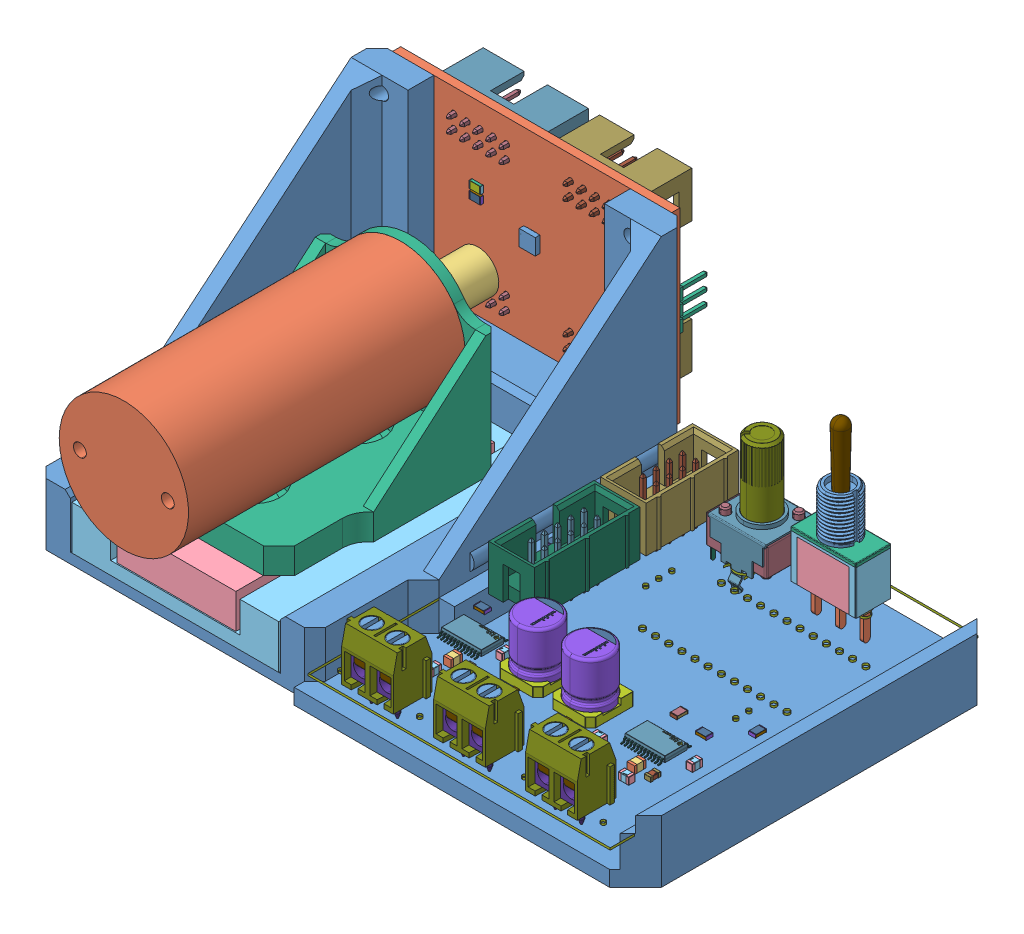
SolidWorks assembly 07_01_00-pidgeon_drive_testing_rig, configuration Default. Lengths in mm.
Overall size (121 48 89.69).
399 component instances, 88 part files, 20 mates.
Components (placement in the parent):
- 07_01_01-encoder_PCB_bracket-1: 07_01_01-encoder_PCB_bracket [Default] at (-11.5568 16.63 42.3747) size (121 48 71)
- 07_01_02-encoder_PCB.step-1: 07_01_02-encoder_PCB.step [Default] at (-14.5568 13.63 42.3747) size (54 36 12.1)
  - Board.step-1: Board.step [Default] at origin size (54 36 1.59)
    - Open CASCADE STEP translator 7.5 1.1.1.step-1: Open CASCADE STEP translator 7.5 1.1.1.step [Default] at (0 0 -1.59) size (54 36 1.59)
  - U2.step-1: U2.step [Default] at origin size (4 3.5 1)
    - 6290729904.step-1: 6290729904.step [Default] at (17.25 17.25 -2.59) size (4 3.5 1)
      - Extruded.step-1: Extruded.step [Default] at origin size (4 3.5 1)
  - R8.step-1: R8.step [Default] at origin size (2.2 1.45 0.7)
    - 6290729184.step-1: 6290729184.step [Default] at (47 19.5 -2.29) size (1.4 1.45 0.7)
      - Extruded-0.step-1: Extruded-0.step [Default] at origin size (1.4 1.45 0.7)
    - 6290729024.step-1: 6290729024.step [Default] at (46.1 19.5 -2.29) size (0.4 1.45 0.7)
      - Extruded-1.step-1: Extruded-1.step [Default] at origin size (0.4 1.45 0.7)
    - 6290729024.step-2: 6290729024.step [Default] at (47.9 19.5 -2.29) size (0.4 1.45 0.7)
      - Extruded-1.step-1: Extruded-1.step [Default] at origin size (0.4 1.45 0.7)
  - R7.step-1: R7.step [Default] at origin size (2.2 1.45 0.7)
    - 6290729184.step-1: 6290729184.step [Default] at (47 17.25 -2.29) size (1.4 1.45 0.7)
      - Extruded-0.step-1: Extruded-0.step [Default] at origin size (1.4 1.45 0.7)
    - 6290729024.step-1: 6290729024.step [Default] at (46.1 17.25 -2.29) size (0.4 1.45 0.7)
      - Extruded-1.step-1: Extruded-1.step [Default] at origin size (0.4 1.45 0.7)
    - 6290729024.step-2: 6290729024.step [Default] at (47.9 17.25 -2.29) size (0.4 1.45 0.7)
      - Extruded-1.step-1: Extruded-1.step [Default] at origin size (0.4 1.45 0.7)
  - R6.step-1: R6.step [Default] at origin size (2.2 1.45 0.7)
    - 6290729184.step-1: 6290729184.step [Default] at (47 15 -2.29) size (1.4 1.45 0.7)
      - Extruded-0.step-1: Extruded-0.step [Default] at origin size (1.4 1.45 0.7)
    - 6290729024.step-1: 6290729024.step [Default] at (46.1 15 -2.29) size (0.4 1.45 0.7)
      - Extruded-1.step-1: Extruded-1.step [Default] at origin size (0.4 1.45 0.7)
    - 6290729024.step-2: 6290729024.step [Default] at (47.9 15 -2.29) size (0.4 1.45 0.7)
      - Extruded-1.step-1: Extruded-1.step [Default] at origin size (0.4 1.45 0.7)
  - P5.step-1: P5.step [Default] at origin size (2.54 7.62 10.92)
    - TSW-103-07-X-S.step-1: TSW-103-07-X-S.step [Default] at (50.7499 18.0199 -1.59) x (0 1 0) z (-1 0 0) size (7.62 10.92 2.54)
  - D3.step-1: D3.step [Default] at origin size (2 1.25 0.8)
    - Diode_Wurth_Electronics_150080SS75000_eec.step-1: Diode_Wurth_Electronics_150080SS75000_eec.step [Default] at (42.5 19.5 -1.59) x (-1 0 0) z (0 0 -1) size (2 1.25 0.8)
      - base.step-1: base.step [Default] at (0.8 0 0) x (-1 0 0) z (0 0 1) size (0.4 1 0.3)
      - cover.step-1: cover.step [Default] at (0 0 0.3) size (1.4 1.25 0.5)
      - housing.step-1: housing.step [Default] at origin size (2 1.25 0.3)
      - marking.step-1: marking.step [Default] at (-0.8 0.525 0.26) size (0.4 0.48 0.04)
      - marking.step-2: marking.step [Default] at (-0.8 -0.525 0.3) x (1 0 0) z (0 0 -1) size (0.4 0.48 0.04)
      - base_2.step-1: base_2.step [Default] at (-0.8 0 0) size (0.4 1 0.3)
      - Mark2.step-1: Mark2.step [Default] at (-0.2 0 0.04) x (-1 0 0) z (0 0 -1) size (0.4 0.46 0)
  - D2.step-1: D2.step [Default] at origin size (2 1.25 0.8)
    - Diode_Wurth_Electronics_150080SS75000_eec.step-1: Diode_Wurth_Electronics_150080SS75000_eec.step [Default] at (42.5 17.25 -1.59) x (-1 0 0) z (0 0 -1) size (2 1.25 0.8)
      - base.step-1: base.step [Default] at (0.8 0 0) x (-1 0 0) z (0 0 1) size (0.4 1 0.3)
      - cover.step-1: cover.step [Default] at (0 0 0.3) size (1.4 1.25 0.5)
      - housing.step-1: housing.step [Default] at origin size (2 1.25 0.3)
      - marking.step-1: marking.step [Default] at (-0.8 0.525 0.26) size (0.4 0.48 0.04)
      - marking.step-2: marking.step [Default] at (-0.8 -0.525 0.3) x (1 0 0) z (0 0 -1) size (0.4 0.48 0.04)
      - base_2.step-1: base_2.step [Default] at (-0.8 0 0) size (0.4 1 0.3)
      - Mark2.step-1: Mark2.step [Default] at (-0.2 0 0.04) x (-1 0 0) z (0 0 -1) size (0.4 0.46 0)
  - D1.step-1: D1.step [Default] at origin size (2 1.25 0.8)
    - Diode_Wurth_Electronics_150080SS75000_eec.step-1: Diode_Wurth_Electronics_150080SS75000_eec.step [Default] at (42.5 15 -1.59) x (-1 0 0) z (0 0 -1) size (2 1.25 0.8)
      - base.step-1: base.step [Default] at (0.8 0 0) x (-1 0 0) z (0 0 1) size (0.4 1 0.3)
      - cover.step-1: cover.step [Default] at (0 0 0.3) size (1.4 1.25 0.5)
      - housing.step-1: housing.step [Default] at origin size (2 1.25 0.3)
      - marking.step-1: marking.step [Default] at (-0.8 0.525 0.26) size (0.4 0.48 0.04)
      - marking.step-2: marking.step [Default] at (-0.8 -0.525 0.3) x (1 0 0) z (0 0 -1) size (0.4 0.48 0.04)
      - base_2.step-1: base_2.step [Default] at (-0.8 0 0) size (0.4 1 0.3)
      - Mark2.step-1: Mark2.step [Default] at (-0.2 0 0.04) x (-1 0 0) z (0 0 -1) size (0.4 0.46 0)
  - C4.step-1: C4.step [Default] at origin size (1.25 2 0.88)
    - Cap_KEMET_C0805C472J3HAC_eec.step-1: Cap_KEMET_C0805C472J3HAC_eec.step [Default] at (25.6247 12.75 -1.59) x (0 -1 0) z (0 0 -1) size (1 1.15 0.78)
    - Cap_KEMET_C0805C472J3HAC_eec-2.step-1: Cap_KEMET_C0805C472J3HAC_eec-2.step [Default] at (25.6247 12.75 -1.59) x (0 -1 0) z (0 0 -1) size (2 1.25 0.88)
    - Cap_KEMET_C0805C472J3HAC_eec-3.step-1: Cap_KEMET_C0805C472J3HAC_eec-3.step [Default] at (25.6247 12.75 -1.59) x (0 -1 0) z (0 0 -1) size (0.59 0.12 0)
  - U4.step-1: U4.step [Default] at origin size (2.8 2.9 1.45)
    - IC_Microchip_MIC7300YM5-TR_eec.step-1: IC_Microchip_MIC7300YM5-TR_eec.step [Default] at (29.5 12.5 -1.59) x (0 -1 0) z (0 0 -1) size (2.9 2.8 1.45)
      - IC_BODY.step-1: IC_BODY.step [Default] at (0 0 0.15) x (0 -1 0) z (0 0 1) size (1.6 2.9 1.3)
      - IC_LEG.step-1: IC_LEG.step [Default] at (1.15 1.4 0) x (0 -1 0) z (-1 0 0) size (0.6 0.86 0.4)
      - IC_LEG.step-2: IC_LEG.step [Default] at (0.2 1.4 0) x (0 -1 0) z (-1 0 0) size (0.6 0.86 0.4)
      - IC_LEG.step-3: IC_LEG.step [Default] at (-0.75 1.4 0) x (0 -1 0) z (-1 0 0) size (0.6 0.86 0.4)
      - circle.step-1: circle.step [Default] at (0.9954 0.3904 1.451) x (1 0 0) z (0 0 -1) size (0.4 0.4 0)
      - IC_LEG_MIR1.step-1: IC_LEG_MIR1.step [Default] at (1.15 -1.4 0) x (0 1 0) z (1 0 0) size (0.6 0.86 0.4)
      - IC_LEG_MIR1.step-2: IC_LEG_MIR1.step [Default] at (-0.75 -1.4 0) x (0 1 0) z (1 0 0) size (0.6 0.86 0.4)
      - Microchip logo.step-1: Microchip logo.step [Default] at (-1.0431 -0.33 1.4496) x (0 -1 0) z (0 0 1) size (0.4 0.39 0)
  - R5.step-1: R5.step [Default] at origin size (2.2 1.45 0.6)
    - 6290728304.step-1: 6290728304.step [Default] at (4.75 23.25 -2.19) size (1.4 1.45 0.6)
      - Extruded-4.step-1: Extruded-4.step [Default] at origin size (1.4 1.45 0.6)
    - 6290728144.step-1: 6290728144.step [Default] at (3.85 23.25 -2.19) size (0.4 1.45 0.6)
      - Extruded-5.step-1: Extruded-5.step [Default] at origin size (0.4 1.45 0.6)
    - 6290728144.step-2: 6290728144.step [Default] at (5.65 23.25 -2.19) size (0.4 1.45 0.6)
      - Extruded-5.step-1: Extruded-5.step [Default] at origin size (0.4 1.45 0.6)
  - R4.step-1: R4.step [Default] at origin size (2.2 1.45 0.6)
    - 6290728304.step-1: 6290728304.step [Default] at (15 23.25 -2.19) size (1.4 1.45 0.6)
      - Extruded-4.step-1: Extruded-4.step [Default] at origin size (1.4 1.45 0.6)
    - 6290728144.step-1: 6290728144.step [Default] at (14.1 23.25 -2.19) size (0.4 1.45 0.6)
      - Extruded-5.step-1: Extruded-5.step [Default] at origin size (0.4 1.45 0.6)
    - 6290728144.step-2: 6290728144.step [Default] at (15.9 23.25 -2.19) size (0.4 1.45 0.6)
      - Extruded-5.step-1: Extruded-5.step [Default] at origin size (0.4 1.45 0.6)
  - R3.step-1: R3.step [Default] at origin size (2.2 1.45 0.6)
    - 6290728304.step-1: 6290728304.step [Default] at (9.25 23.25 -2.19) size (1.4 1.45 0.6)
      - Extruded-4.step-1: Extruded-4.step [Default] at origin size (1.4 1.45 0.6)
    - 6290728144.step-1: 6290728144.step [Default] at (10.15 23.25 -2.19) size (0.4 1.45 0.6)
      - Extruded-5.step-1: Extruded-5.step [Default] at origin size (0.4 1.45 0.6)
    - 6290728144.step-2: 6290728144.step [Default] at (8.35 23.25 -2.19) size (0.4 1.45 0.6)
      - Extruded-5.step-1: Extruded-5.step [Default] at origin size (0.4 1.45 0.6)
  - R2.step-1: R2.step [Default] at origin size (2.2 1.35 0.6)
    - 6361395456.step-1: 6361395456.step [Default] at (16.5 21.75 0) size (2.2 1.35 0.6)
      - Terminal.step-1: Terminal.step [Default] at (-1.1 -0.675 0) size (0.15 1.35 0.6)
        - Open CASCADE STEP translator 6.8 7.2.1.step-1: Open CASCADE STEP translator 6.8 7.2.1.step [Default] at origin size (0.15 1.35 0.6)
      - Terminal.step-2: Terminal.step [Default] at (1.1 0.675 0) x (-1 0 0) z (0 0 1) size (0.15 1.35 0.6)
        - Open CASCADE STEP translator 6.8 7.2.1.step-1: Open CASCADE STEP translator 6.8 7.2.1.step [Default] at origin size (0.15 1.35 0.6)
      - Mid_Body.step-1: Mid_Body.step [Default] at (-1.1 -0.675 0) size (2.08 1.35 0.48)
      - Mark.step-1: Mark.step [Default] at (-0.95 -0.675 0.54) size (1.9 1.35 0.06)
  - R1.step-1: R1.step [Default] at origin size (2.2 1.35 0.6)
    - 6361394336.step-1: 6361394336.step [Default] at (16.5 20 0) x (-1 0 0) z (0 0 1) size (2.2 1.35 0.6)
      - Terminal-1.step-1: Terminal-1.step [Default] at (-1.1 -0.675 0) size (0.15 1.35 0.6)
        - Open CASCADE STEP translator 6.8 7.2.1-6.step-1: Open CASCADE STEP translator 6.8 7.2.1-6.step [Default] at origin size (0.15 1.35 0.6)
      - Terminal-1.step-2: Terminal-1.step [Default] at (1.1 0.675 0) x (-1 0 0) z (0 0 1) size (0.15 1.35 0.6)
        - Open CASCADE STEP translator 6.8 7.2.1-6.step-1: Open CASCADE STEP translator 6.8 7.2.1-6.step [Default] at origin size (0.15 1.35 0.6)
      - Mid_Body-7.step-1: Mid_Body-7.step [Default] at (-1.1 -0.675 0) size (2.08 1.35 0.48)
      - Mark-8.step-1: Mark-8.step [Default] at (-0.95 -0.675 0.54) size (1.9 1.35 0.06)
  - P4.step-1: P4.step [Default] at origin size (17.82 9.18 12.1)
    - 61200821621.step-1: 61200821621.step [Default] at (38.2501 30.2499 -6.29) x (1 0 0) z (0 0 -1) size (17.82 9.17 12.1)
      - 6120xx21621_PIN.step-1: 6120xx21621_PIN.step [Default] at (-0.405 1.27 -1.875) size (0.64 0.64 11.6)
      - 6120xx21621_PIN.step-2: 6120xx21621_PIN.step [Default] at (-0.405 -1.27 -1.875) size (0.64 0.64 11.6)
      - 6120xx21621_PIN.step-3: 6120xx21621_PIN.step [Default] at (2.135 -1.27 -1.875) size (0.64 0.64 11.6)
      - 6120xx21621_PIN.step-4: 6120xx21621_PIN.step [Default] at (4.675 -1.27 -1.875) size (0.64 0.64 11.6)
      - 6120xx21621_PIN.step-5: 6120xx21621_PIN.step [Default] at (2.135 1.27 -1.875) size (0.64 0.64 11.6)
      - 6120xx21621_PIN.step-6: 6120xx21621_PIN.step [Default] at (4.675 1.27 -1.875) size (0.64 0.64 11.6)
      - 6120xx21621_PIN.step-7: 6120xx21621_PIN.step [Default] at (7.215 -1.27 -1.875) size (0.64 0.64 11.6)
      - 6120xx21621_PIN.step-8: 6120xx21621_PIN.step [Default] at (7.215 1.27 -1.875) size (0.64 0.64 11.6)
      - 61200821621-9.step-1: 61200821621-9.step [Default] at origin size (17.82 9.17 9.1)
  - P3.step-1: P3.step [Default] at origin size (20.36 9.18 12.1)
    - 61201021621.step-1: 61201021621.step [Default] at (17.0001 30.2499 -6.29) x (1 0 0) z (0 0 -1) size (20.36 9.17 12.1)
      - 6120xx21621_PIN-10.step-1: 6120xx21621_PIN-10.step [Default] at (-1.675 1.27 -1.875) size (0.64 0.64 11.6)
      - 6120xx21621_PIN-10.step-2: 6120xx21621_PIN-10.step [Default] at (-1.675 -1.27 -1.875) size (0.64 0.64 11.6)
      - 6120xx21621_PIN-10.step-3: 6120xx21621_PIN-10.step [Default] at (0.865 -1.27 -1.875) size (0.64 0.64 11.6)
      - 6120xx21621_PIN-10.step-4: 6120xx21621_PIN-10.step [Default] at (3.405 -1.27 -1.875) size (0.64 0.64 11.6)
      - 6120xx21621_PIN-10.step-5: 6120xx21621_PIN-10.step [Default] at (0.865 1.27 -1.875) size (0.64 0.64 11.6)
      - 6120xx21621_PIN-10.step-6: 6120xx21621_PIN-10.step [Default] at (3.405 1.27 -1.875) size (0.64 0.64 11.6)
      - 6120xx21621_PIN-10.step-7: 6120xx21621_PIN-10.step [Default] at (5.945 -1.27 -1.875) size (0.64 0.64 11.6)
      - 6120xx21621_PIN-10.step-8: 6120xx21621_PIN-10.step [Default] at (5.945 1.27 -1.875) size (0.64 0.64 11.6)
      - 6120xx21621_PIN-10.step-9: 6120xx21621_PIN-10.step [Default] at (8.485 -1.27 -1.875) size (0.64 0.64 11.6)
      - 6120xx21621_PIN-10.step-10: 6120xx21621_PIN-10.step [Default] at (8.485 1.27 -1.875) size (0.64 0.64 11.6)
      - 61201021621-11.step-1: 61201021621-11.step [Default] at origin size (20.36 9.17 9.1)
  - P2.step-1: P2.step [Default] at origin size (17.82 9.18 12.1)
    - 61200821621.step-1: 61200821621.step [Default] at (38.2501 4.9999 -6.29) x (1 0 0) z (0 0 -1) size (17.82 9.17 12.1)
      - 6120xx21621_PIN.step-1: 6120xx21621_PIN.step [Default] at (-0.405 1.27 -1.875) size (0.64 0.64 11.6)
      - 6120xx21621_PIN.step-2: 6120xx21621_PIN.step [Default] at (-0.405 -1.27 -1.875) size (0.64 0.64 11.6)
      - 6120xx21621_PIN.step-3: 6120xx21621_PIN.step [Default] at (2.135 -1.27 -1.875) size (0.64 0.64 11.6)
      - 6120xx21621_PIN.step-4: 6120xx21621_PIN.step [Default] at (4.675 -1.27 -1.875) size (0.64 0.64 11.6)
      - 6120xx21621_PIN.step-5: 6120xx21621_PIN.step [Default] at (2.135 1.27 -1.875) size (0.64 0.64 11.6)
      - 6120xx21621_PIN.step-6: 6120xx21621_PIN.step [Default] at (4.675 1.27 -1.875) size (0.64 0.64 11.6)
      - 6120xx21621_PIN.step-7: 6120xx21621_PIN.step [Default] at (7.215 -1.27 -1.875) size (0.64 0.64 11.6)
      - 6120xx21621_PIN.step-8: 6120xx21621_PIN.step [Default] at (7.215 1.27 -1.875) size (0.64 0.64 11.6)
      - 61200821621-9.step-1: 61200821621-9.step [Default] at origin size (17.82 9.17 9.1)
  - P1.step-1: P1.step [Default] at origin size (20.36 9.18 12.1)
    - 61201021621.step-1: 61201021621.step [Default] at (17.0001 4.9999 -6.29) x (1 0 0) z (0 0 -1) size (20.36 9.17 12.1)
      - 6120xx21621_PIN-10.step-1: 6120xx21621_PIN-10.step [Default] at (-1.675 1.27 -1.875) size (0.64 0.64 11.6)
      - 6120xx21621_PIN-10.step-2: 6120xx21621_PIN-10.step [Default] at (-1.675 -1.27 -1.875) size (0.64 0.64 11.6)
      - 6120xx21621_PIN-10.step-3: 6120xx21621_PIN-10.step [Default] at (0.865 -1.27 -1.875) size (0.64 0.64 11.6)
      - 6120xx21621_PIN-10.step-4: 6120xx21621_PIN-10.step [Default] at (3.405 -1.27 -1.875) size (0.64 0.64 11.6)
      - 6120xx21621_PIN-10.step-5: 6120xx21621_PIN-10.step [Default] at (0.865 1.27 -1.875) size (0.64 0.64 11.6)
      - 6120xx21621_PIN-10.step-6: 6120xx21621_PIN-10.step [Default] at (3.405 1.27 -1.875) size (0.64 0.64 11.6)
      - 6120xx21621_PIN-10.step-7: 6120xx21621_PIN-10.step [Default] at (5.945 -1.27 -1.875) size (0.64 0.64 11.6)
      - 6120xx21621_PIN-10.step-8: 6120xx21621_PIN-10.step [Default] at (5.945 1.27 -1.875) size (0.64 0.64 11.6)
      - 6120xx21621_PIN-10.step-9: 6120xx21621_PIN-10.step [Default] at (8.485 -1.27 -1.875) size (0.64 0.64 11.6)
      - 6120xx21621_PIN-10.step-10: 6120xx21621_PIN-10.step [Default] at (8.485 1.27 -1.875) size (0.64 0.64 11.6)
      - 61201021621-11.step-1: 61201021621-11.step [Default] at origin size (20.36 9.17 9.1)
  - C3.step-1: C3.step [Default] at origin size (1.35 2.1 0.7)
    - 6290729744.step-1: 6290729744.step [Default] at (30 17.75 -2.29) size (1.35 1.2 0.7)
      - Extruded-12.step-1: Extruded-12.step [Default] at origin size (1.35 1.2 0.7)
    - 6290729584.step-1: 6290729584.step [Default] at (30 16.925 -2.29) size (1.35 0.45 0.7)
      - Extruded-13.step-1: Extruded-13.step [Default] at origin size (1.35 0.45 0.7)
    - 6290729584.step-2: 6290729584.step [Default] at (30 18.575 -2.29) size (1.35 0.45 0.7)
      - Extruded-13.step-1: Extruded-13.step [Default] at origin size (1.35 0.45 0.7)
  - C2.step-1: C2.step [Default] at origin size (1.25 2 0.88)
    - Cap_KEMET_C0805C472J3HAC_eec.step-1: Cap_KEMET_C0805C472J3HAC_eec.step [Default] at (2.5 16.25 -1.59) x (0 1 0) z (0 0 -1) size (1 1.15 0.78)
    - Cap_KEMET_C0805C472J3HAC_eec-2.step-1: Cap_KEMET_C0805C472J3HAC_eec-2.step [Default] at (2.5 16.25 -1.59) x (0 1 0) z (0 0 -1) size (2 1.25 0.88)
    - Cap_KEMET_C0805C472J3HAC_eec-3.step-1: Cap_KEMET_C0805C472J3HAC_eec-3.step [Default] at (2.5 16.25 -1.59) x (0 1 0) z (0 0 -1) size (0.59 0.12 0)
  - C1.step-1: C1.step [Default] at origin size (1.25 2 0.88)
    - Cap_KEMET_C0805C472J3HAC_eec.step-1: Cap_KEMET_C0805C472J3HAC_eec.step [Default] at (12.75 16.25 -1.59) x (0 1 0) z (0 0 -1) size (1 1.15 0.78)
    - Cap_KEMET_C0805C472J3HAC_eec-2.step-1: Cap_KEMET_C0805C472J3HAC_eec-2.step [Default] at (12.75 16.25 -1.59) x (0 1 0) z (0 0 -1) size (2 1.25 0.88)
    - Cap_KEMET_C0805C472J3HAC_eec-3.step-1: Cap_KEMET_C0805C472J3HAC_eec-3.step [Default] at (12.75 16.25 -1.59) x (0 1 0) z (0 0 -1) size (0.59 0.12 0)
  - U3.step-1: U3.step [Default] at origin size (5 6.42 1)
    - PW0016AakaMTC16.step-1: PW0016AakaMTC16.step [Default] at (6.9999 17.2499 -2.213) x (-1 0 0) z (0 -1 0) size (5 1 6.42)
      - BODY_MTC16.step-1: BODY_MTC16.step [Default] at origin size (5 0.9 4.4)
      - LEAD_MTC16.step-1: LEAD_MTC16.step [Default] at (2.275 -0.3725 -2.6) x (-1 0 0) z (0 0 -1) size (0.24 0.62 1.01)
      - LEAD_MTC16.step-2: LEAD_MTC16.step [Default] at (1.625 -0.3725 -2.6) x (-1 0 0) z (0 0 -1) size (0.24 0.62 1.01)
      - LEAD_MTC16.step-3: LEAD_MTC16.step [Default] at (0.975 -0.3725 -2.6) x (-1 0 0) z (0 0 -1) size (0.24 0.62 1.01)
      - LEAD_MTC16.step-4: LEAD_MTC16.step [Default] at (0.325 -0.3725 -2.6) x (-1 0 0) z (0 0 -1) size (0.24 0.62 1.01)
      - LEAD_MTC16.step-5: LEAD_MTC16.step [Default] at (-0.325 -0.3725 -2.6) x (-1 0 0) z (0 0 -1) size (0.24 0.62 1.01)
      - LEAD_MTC16.step-6: LEAD_MTC16.step [Default] at (-0.975 -0.3725 -2.6) x (-1 0 0) z (0 0 -1) size (0.24 0.62 1.01)
      - LEAD_MTC16.step-7: LEAD_MTC16.step [Default] at (-1.625 -0.3725 -2.6) x (-1 0 0) z (0 0 -1) size (0.24 0.62 1.01)
      - LEAD_MTC16.step-8: LEAD_MTC16.step [Default] at (-2.275 -0.3725 -2.6) x (-1 0 0) z (0 0 -1) size (0.24 0.62 1.01)
      - LEAD_MTC16.step-9: LEAD_MTC16.step [Default] at (2.275 -0.3725 2.6) size (0.24 0.62 1.01)
      - LEAD_MTC16.step-10: LEAD_MTC16.step [Default] at (1.625 -0.3725 2.6) size (0.24 0.62 1.01)
      - LEAD_MTC16.step-11: LEAD_MTC16.step [Default] at (0.975 -0.3725 2.6) size (0.24 0.62 1.01)
      - LEAD_MTC16.step-12: LEAD_MTC16.step [Default] at (0.325 -0.3725 2.6) size (0.24 0.62 1.01)
      - LEAD_MTC16.step-13: LEAD_MTC16.step [Default] at (-0.325 -0.3725 2.6) size (0.24 0.62 1.01)
      - LEAD_MTC16.step-14: LEAD_MTC16.step [Default] at (-0.975 -0.3725 2.6) size (0.24 0.62 1.01)
      - LEAD_MTC16.step-15: LEAD_MTC16.step [Default] at (-1.625 -0.3725 2.6) size (0.24 0.62 1.01)
      - LEAD_MTC16.step-16: LEAD_MTC16.step [Default] at (-2.275 -0.3725 2.6) size (0.24 0.62 1.01)
  - U1.step-1: U1.step [Default] at origin size (3.1 3.1 0.94)
    - 6361392256.step-1: 6361392256.step [Default] at (27 18 0) size (3.1 3.1 0.94)
- 07_01_04-motor-1: 07_01_04-motor [Default] at (12.4806 31.63 121.354) x (1 0 0) z (0 0 -1) size (25 25 66.5)
- 07_01_03-magnet_holder-1: 07_01_03-magnet_holder [Default] at (12.4806 31.63 64.854) x (-0.768506 0.639842 0) z (-0.639842 -0.768506 0) size (8 12 8)
- 07_01_05-carriage_moving-1: 07_01_05-carriage_moving [Default] at (0.9432 6.13 111.154) size (23 6.7 50)
- 07_01_06-carriage_static-1: 07_01_06-carriage_static [Default] at (-7.5568 3.63 111.3747) size (40 8.5 60)
- 07_01_07-motor_mount-1: 07_01_07-motor_mount [Default] at (12.4806 12.83 96.154) x (-1 0 0) z (0 0 -1) size (33 31.3 40)
- 07_01_08-pidgeon_drive_PCB.STEP-1: 07_01_08-pidgeon_drive_PCB.STEP [Default] at (17.0432 10.63 -62.1104) x (0 0 1) z (0 1 0) size (71.12 58.42 35.31)
  - Board.step.STEP-1: Board.step.STEP [Default] at origin size (71.12 58.42 0.41)
    - Open CASCADE STEP translator 7.5 1.1.1.step.STEP-1: Open CASCADE STEP translator 7.5 1.1.1.step.STEP [Default] at (0 0 -0.4115) size (71.12 58.42 0.41)
  - R8.step.STEP-1: R8.step.STEP [Default] at origin size (2.1 1.35 0.6)
    - 6599227264.step.STEP-1: 6599227264.step.STEP [Default] at (132.32 27.41 0) size (2.1 1.35 0.6)
      - Terminal.step.STEP-1: Terminal.step.STEP [Default] at (-1.05 -0.675 0) size (0.15 1.35 0.6)
        - Open CASCADE STEP translator 6.8 3.2.1.step.STEP-1: Open CASCADE STEP translator 6.8 3.2.1.step.STEP [Default] at origin size (0.15 1.35 0.6)
      - Terminal.step.STEP-2: Terminal.step.STEP [Default] at (1.05 0.675 0) x (-1 0 0) z (0 0 1) size (0.15 1.35 0.6)
        - Open CASCADE STEP translator 6.8 3.2.1.step.STEP-1: Open CASCADE STEP translator 6.8 3.2.1.step.STEP [Default] at origin size (0.15 1.35 0.6)
      - Mid_Body.step.STEP-1: Mid_Body.step.STEP [Default] at (-1.05 -0.675 0) size (1.98 1.35 0.48)
      - Mark.step.STEP-1: Mark.step.STEP [Default] at (-0.9 -0.675 0.54) size (1.8 1.35 0.06)
  - R7.step.STEP-1: R7.step.STEP [Default] at origin size (2.1 1.35 0.6)
    - 6599227264.step.STEP-1: 6599227264.step.STEP [Default] at (137.77 27.41 0) size (2.1 1.35 0.6)
      - Terminal.step.STEP-1: Terminal.step.STEP [Default] at (-1.05 -0.675 0) size (0.15 1.35 0.6)
        - Open CASCADE STEP translator 6.8 3.2.1.step.STEP-1: Open CASCADE STEP translator 6.8 3.2.1.step.STEP [Default] at origin size (0.15 1.35 0.6)
      - Terminal.step.STEP-2: Terminal.step.STEP [Default] at (1.05 0.675 0) x (-1 0 0) z (0 0 1) size (0.15 1.35 0.6)
        - Open CASCADE STEP translator 6.8 3.2.1.step.STEP-1: Open CASCADE STEP translator 6.8 3.2.1.step.STEP [Default] at origin size (0.15 1.35 0.6)
      - Mid_Body.step.STEP-1: Mid_Body.step.STEP [Default] at (-1.05 -0.675 0) size (1.98 1.35 0.48)
      - Mark.step.STEP-1: Mark.step.STEP [Default] at (-0.9 -0.675 0.54) size (1.8 1.35 0.06)
  - P8.step.STEP-1: P8.step.STEP [Default] at origin size (17.82 9.18 12.1)
    - 61200821621.step.STEP-1: 61200821621.step.STEP [Default] at (116.8401 34.2901 4.7) x (1 0 0) z (0 0 1) size (17.82 9.17 12.1)
      - 6120xx21621_PIN.step.STEP-1: 6120xx21621_PIN.step.STEP [Default] at (-0.405 1.27 -1.875) size (0.64 0.64 11.6)
      - 6120xx21621_PIN.step.STEP-2: 6120xx21621_PIN.step.STEP [Default] at (-0.405 -1.27 -1.875) size (0.64 0.64 11.6)
      - 6120xx21621_PIN.step.STEP-3: 6120xx21621_PIN.step.STEP [Default] at (2.135 -1.27 -1.875) size (0.64 0.64 11.6)
      - 6120xx21621_PIN.step.STEP-4: 6120xx21621_PIN.step.STEP [Default] at (4.675 -1.27 -1.875) size (0.64 0.64 11.6)
      - 6120xx21621_PIN.step.STEP-5: 6120xx21621_PIN.step.STEP [Default] at (2.135 1.27 -1.875) size (0.64 0.64 11.6)
      - 6120xx21621_PIN.step.STEP-6: 6120xx21621_PIN.step.STEP [Default] at (4.675 1.27 -1.875) size (0.64 0.64 11.6)
      - 6120xx21621_PIN.step.STEP-7: 6120xx21621_PIN.step.STEP [Default] at (7.215 -1.27 -1.875) size (0.64 0.64 11.6)
      - 6120xx21621_PIN.step.STEP-8: 6120xx21621_PIN.step.STEP [Default] at (7.215 1.27 -1.875) size (0.64 0.64 11.6)
      - 61200821621-0.step.STEP-1: 61200821621-0.step.STEP [Default] at origin size (17.82 9.17 9.1)
  - R4.step.STEP-1: R4.step.STEP [Default] at origin size (11.27 12.64 24.3)
    - Res_Bourns_PTV09A-4225F-B103_eec.step.STEP-1: Res_Bourns_PTV09A-4225F-B103_eec.step.STEP [Default] at (114.1 49.5 0) size (11.27 12.64 24.3)
      - body.step.STEP-1: body.step.STEP [Default] at origin size (9.41 11.82 8)
      - shell.step.STEP-1: shell.step.STEP [Default] at origin size (11.27 11 11.4)
      - pins.step.STEP-1: pins.step.STEP [Default] at origin size (6.5 3.25 6.8)
      - shaft.step.STEP-1: shaft.step.STEP [Default] at origin size (6 6 14.57)
      - logo.step.STEP-1: logo.step.STEP [Default] at (-5 0 6.8) x (0 -1 0) z (-1 0 0) size (8.73 2.81 2.33)
  - SW1.step.STEP-1: SW1.step.STEP [Default] at origin size (7.24 12.7 35.31)
    - Switch_TE_Connectivity_A101SYCB04_eec.step.STEP-1: Switch_TE_Connectivity_A101SYCB04_eec.step.STEP [Default] at (113.8 64.4 0) x (0 -1 0) z (0 0 1) size (12.7 7.24 35.31)
      - 1.step.STEP-1: 1.step.STEP [Default] at (0 0 10.4399) x (-1 0 0) z (0 0 1) size (12.7 7.24 35.31)
        - 1-1.step.STEP-1: 1-1.step.STEP [Default] at origin size (2.92 2.92 12.18)
        - 2.step.STEP-1: 2.step.STEP [Default] at origin size (6.92 7.24 8.66)
        - 3.step.STEP-1: 3.step.STEP [Default] at origin size (10.16 1.27 4.8)
        - 4.step.STEP-1: 4.step.STEP [Default] at origin size (11.94 3.05 1.55)
        - 5.step.STEP-1: 5.step.STEP [Default] at origin size (10 6.86 8)
        - 6.step.STEP-1: 6.step.STEP [Default] at origin size (12.7 6.86 8.5)
        - c-4-1825136-4-a-3d.step.STEP-1: c-4-1825136-4-a-3d.step.STEP [Default] at origin size (12.7 6.86 0.64)
        - TE connectivity Logo 1 (2).step.STEP-1: TE connectivity Logo 1 (2).step.STEP [Default] at (-8.1647 3.33 -1.1849) x (1 0 0) z (0 1 0) size (8.81 6.93 0.1)
  - R1.step.STEP-1: R1.step.STEP [Default] at origin size (1.35 2.1 0.6)
    - 6599213744.step.STEP-1: 6599213744.step.STEP [Default] at (149.9 74.1 0) x (0 1 0) z (0 0 1) size (2.1 1.35 0.6)
      - Terminal-1.step.STEP-1: Terminal-1.step.STEP [Default] at (-1.05 -0.675 0) size (0.15 1.35 0.6)
        - Open CASCADE STEP translator 6.8 3.2.1-2.step.STEP-1: Open CASCADE STEP translator 6.8 3.2.1-2.step.STEP [Default] at origin size (0.15 1.35 0.6)
      - Terminal-1.step.STEP-2: Terminal-1.step.STEP [Default] at (1.05 0.675 0) x (-1 0 0) z (0 0 1) size (0.15 1.35 0.6)
        - Open CASCADE STEP translator 6.8 3.2.1-2.step.STEP-1: Open CASCADE STEP translator 6.8 3.2.1-2.step.STEP [Default] at origin size (0.15 1.35 0.6)
      - Mid_Body-3.step.STEP-1: Mid_Body-3.step.STEP [Default] at (-1.05 -0.675 0) size (1.98 1.35 0.48)
      - Mark-4.step.STEP-1: Mark-4.step.STEP [Default] at (-0.9 -0.675 0.54) size (1.8 1.35 0.06)
  - R2.step.STEP-1: R2.step.STEP [Default] at origin size (2.1 1.35 0.6)
    - 6599216544.step.STEP-1: 6599216544.step.STEP [Default] at (148.9 68.2 0) x (1 0 0) z (0 0 1) size (2.1 1.35 0.6)
      - Terminal-2.step.STEP-1: Terminal-2.step.STEP [Default] at (-1.05 -0.675 0) size (0.15 1.35 0.6)
        - Open CASCADE STEP translator 6.8 3.2.1-5.step.STEP-1: Open CASCADE STEP translator 6.8 3.2.1-5.step.STEP [Default] at origin size (0.15 1.35 0.6)
      - Terminal-2.step.STEP-2: Terminal-2.step.STEP [Default] at (1.05 0.675 0) x (-1 0 0) z (0 0 1) size (0.15 1.35 0.6)
        - Open CASCADE STEP translator 6.8 3.2.1-5.step.STEP-1: Open CASCADE STEP translator 6.8 3.2.1-5.step.STEP [Default] at origin size (0.15 1.35 0.6)
      - Mid_Body-6.step.STEP-1: Mid_Body-6.step.STEP [Default] at (-1.05 -0.675 0) size (1.98 1.35 0.48)
      - Mark-7.step.STEP-1: Mark-7.step.STEP [Default] at (-0.9 -0.675 0.54) size (1.8 1.35 0.06)
  - R6.step.STEP-1: R6.step.STEP [Default] at origin size (2.1 1.35 0.6)
    - 6599227264.step.STEP-1: 6599227264.step.STEP [Default] at (144.4 78.9 0) size (2.1 1.35 0.6)
      - Terminal.step.STEP-1: Terminal.step.STEP [Default] at (-1.05 -0.675 0) size (0.15 1.35 0.6)
        - Open CASCADE STEP translator 6.8 3.2.1.step.STEP-1: Open CASCADE STEP translator 6.8 3.2.1.step.STEP [Default] at origin size (0.15 1.35 0.6)
      - Terminal.step.STEP-2: Terminal.step.STEP [Default] at (1.05 0.675 0) x (-1 0 0) z (0 0 1) size (0.15 1.35 0.6)
        - Open CASCADE STEP translator 6.8 3.2.1.step.STEP-1: Open CASCADE STEP translator 6.8 3.2.1.step.STEP [Default] at origin size (0.15 1.35 0.6)
      - Mid_Body.step.STEP-1: Mid_Body.step.STEP [Default] at (-1.05 -0.675 0) size (1.98 1.35 0.48)
      - Mark.step.STEP-1: Mark.step.STEP [Default] at (-0.9 -0.675 0.54) size (1.8 1.35 0.06)
  - R3.step.STEP-1: R3.step.STEP [Default] at origin size (1.35 2.1 0.6)
    - 6599213744.step.STEP-1: 6599213744.step.STEP [Default] at (150.1 39.7 0) x (0 1 0) z (0 0 1) size (2.1 1.35 0.6)
      - Terminal-1.step.STEP-1: Terminal-1.step.STEP [Default] at (-1.05 -0.675 0) size (0.15 1.35 0.6)
        - Open CASCADE STEP translator 6.8 3.2.1-2.step.STEP-1: Open CASCADE STEP translator 6.8 3.2.1-2.step.STEP [Default] at origin size (0.15 1.35 0.6)
      - Terminal-1.step.STEP-2: Terminal-1.step.STEP [Default] at (1.05 0.675 0) x (-1 0 0) z (0 0 1) size (0.15 1.35 0.6)
        - Open CASCADE STEP translator 6.8 3.2.1-2.step.STEP-1: Open CASCADE STEP translator 6.8 3.2.1-2.step.STEP [Default] at origin size (0.15 1.35 0.6)
      - Mid_Body-3.step.STEP-1: Mid_Body-3.step.STEP [Default] at (-1.05 -0.675 0) size (1.98 1.35 0.48)
      - Mark-4.step.STEP-1: Mark-4.step.STEP [Default] at (-0.9 -0.675 0.54) size (1.8 1.35 0.06)
  - R5.step.STEP-1: R5.step.STEP [Default] at origin size (1.35 2.1 0.6)
    - 6599213744.step.STEP-1: 6599213744.step.STEP [Default] at (150.3 31.6 0) x (0 1 0) z (0 0 1) size (2.1 1.35 0.6)
      - Terminal-1.step.STEP-1: Terminal-1.step.STEP [Default] at (-1.05 -0.675 0) size (0.15 1.35 0.6)
        - Open CASCADE STEP translator 6.8 3.2.1-2.step.STEP-1: Open CASCADE STEP translator 6.8 3.2.1-2.step.STEP [Default] at origin size (0.15 1.35 0.6)
      - Terminal-1.step.STEP-2: Terminal-1.step.STEP [Default] at (1.05 0.675 0) x (-1 0 0) z (0 0 1) size (0.15 1.35 0.6)
        - Open CASCADE STEP translator 6.8 3.2.1-2.step.STEP-1: Open CASCADE STEP translator 6.8 3.2.1-2.step.STEP [Default] at origin size (0.15 1.35 0.6)
      - Mid_Body-3.step.STEP-1: Mid_Body-3.step.STEP [Default] at (-1.05 -0.675 0) size (1.98 1.35 0.48)
      - Mark-4.step.STEP-1: Mark-4.step.STEP [Default] at (-0.9 -0.675 0.54) size (1.8 1.35 0.06)
  - P6.step.STEP-1: P6.step.STEP [Default] at origin size (20.36 9.18 12.1)
    - 61201021621.step.STEP-1: 61201021621.step.STEP [Default] at (137.16 34.2901 4.7) x (1 0 0) z (0 0 1) size (20.36 9.17 12.1)
      - 6120xx21621_PIN-8.step.STEP-1: 6120xx21621_PIN-8.step.STEP [Default] at (-1.675 1.27 -1.875) size (0.64 0.64 11.6)
      - 6120xx21621_PIN-8.step.STEP-2: 6120xx21621_PIN-8.step.STEP [Default] at (-1.675 -1.27 -1.875) size (0.64 0.64 11.6)
      - 6120xx21621_PIN-8.step.STEP-3: 6120xx21621_PIN-8.step.STEP [Default] at (0.865 -1.27 -1.875) size (0.64 0.64 11.6)
      - 6120xx21621_PIN-8.step.STEP-4: 6120xx21621_PIN-8.step.STEP [Default] at (3.405 -1.27 -1.875) size (0.64 0.64 11.6)
      - 6120xx21621_PIN-8.step.STEP-5: 6120xx21621_PIN-8.step.STEP [Default] at (0.865 1.27 -1.875) size (0.64 0.64 11.6)
      - 6120xx21621_PIN-8.step.STEP-6: 6120xx21621_PIN-8.step.STEP [Default] at (3.405 1.27 -1.875) size (0.64 0.64 11.6)
      - 6120xx21621_PIN-8.step.STEP-7: 6120xx21621_PIN-8.step.STEP [Default] at (5.945 -1.27 -1.875) size (0.64 0.64 11.6)
      - 6120xx21621_PIN-8.step.STEP-8: 6120xx21621_PIN-8.step.STEP [Default] at (5.945 1.27 -1.875) size (0.64 0.64 11.6)
      - 6120xx21621_PIN-8.step.STEP-9: 6120xx21621_PIN-8.step.STEP [Default] at (8.485 -1.27 -1.875) size (0.64 0.64 11.6)
      - 6120xx21621_PIN-8.step.STEP-10: 6120xx21621_PIN-8.step.STEP [Default] at (8.485 1.27 -1.875) size (0.64 0.64 11.6)
      - 61201021621-9.step.STEP-1: 61201021621-9.step.STEP [Default] at origin size (20.36 9.17 9.1)
  - J3.step.STEP-1: J3.step.STEP [Default] at origin size (7.5 11.2 13.41)
    - 691102710002.step.STEP-1: 691102710002.step.STEP [Default] at (172.72 35.5601 5.01) x (0 1 0) z (0 0 1) size (11.2 7.5 13.41)
      - 691502710002.step.STEP-1: 691502710002.step.STEP [Default] at origin size (11.2 7.5 9.9)
      - 6911027100xx_CAGE.step.STEP-1: 6911027100xx_CAGE.step.STEP [Default] at (2.5 -0.45 -1.75) size (4 4 9.05)
      - 6911027100xx_CAGE.step.STEP-2: 6911027100xx_CAGE.step.STEP [Default] at (-2.5 -0.45 -1.75) size (4 4 9.05)
      - 6911027100xx_PIN.step.STEP-1: 6911027100xx_PIN.step.STEP [Default] at (2.5 -0.45 -0.3503) size (3.9 5.3 2.5)
      - 6911027100xx_PIN.step.STEP-2: 6911027100xx_PIN.step.STEP [Default] at (-2.5 -0.45 -0.3503) size (3.9 5.3 2.5)
      - 6911027100xx_VIS.step.STEP-1: 6911027100xx_VIS.step.STEP [Default] at (2.5 -0.45 4.2) x (0 -1 0) z (0 0 1) size (3.5 3.5 5.31)
      - 6911027100xx_VIS.step.STEP-2: 6911027100xx_VIS.step.STEP [Default] at (-2.5 -0.45 4.2) x (0 -1 0) z (0 0 1) size (3.5 3.5 5.31)
  - J2.step.STEP-1: J2.step.STEP [Default] at origin size (7.5 11.2 13.41)
    - 691102710002.step.STEP-1: 691102710002.step.STEP [Default] at (172.72 53.3401 5.01) x (0 1 0) z (0 0 1) size (11.2 7.5 13.41)
      - 691502710002.step.STEP-1: 691502710002.step.STEP [Default] at origin size (11.2 7.5 9.9)
      - 6911027100xx_CAGE.step.STEP-1: 6911027100xx_CAGE.step.STEP [Default] at (2.5 -0.45 -1.75) size (4 4 9.05)
      - 6911027100xx_CAGE.step.STEP-2: 6911027100xx_CAGE.step.STEP [Default] at (-2.5 -0.45 -1.75) size (4 4 9.05)
      - 6911027100xx_PIN.step.STEP-1: 6911027100xx_PIN.step.STEP [Default] at (2.5 -0.45 -0.3503) size (3.9 5.3 2.5)
      - 6911027100xx_PIN.step.STEP-2: 6911027100xx_PIN.step.STEP [Default] at (-2.5 -0.45 -0.3503) size (3.9 5.3 2.5)
      - 6911027100xx_VIS.step.STEP-1: 6911027100xx_VIS.step.STEP [Default] at (2.5 -0.45 4.2) x (0 -1 0) z (0 0 1) size (3.5 3.5 5.31)
      - 6911027100xx_VIS.step.STEP-2: 6911027100xx_VIS.step.STEP [Default] at (-2.5 -0.45 4.2) x (0 -1 0) z (0 0 1) size (3.5 3.5 5.31)
  - J1.step.STEP-1: J1.step.STEP [Default] at origin size (7.5 11.2 13.41)
    - 691102710002.step.STEP-1: 691102710002.step.STEP [Default] at (172.72 71.1201 5.01) x (0 1 0) z (0 0 1) size (11.2 7.5 13.41)
      - 691502710002.step.STEP-1: 691502710002.step.STEP [Default] at origin size (11.2 7.5 9.9)
      - 6911027100xx_CAGE.step.STEP-1: 6911027100xx_CAGE.step.STEP [Default] at (2.5 -0.45 -1.75) size (4 4 9.05)
      - 6911027100xx_CAGE.step.STEP-2: 6911027100xx_CAGE.step.STEP [Default] at (-2.5 -0.45 -1.75) size (4 4 9.05)
      - 6911027100xx_PIN.step.STEP-1: 6911027100xx_PIN.step.STEP [Default] at (2.5 -0.45 -0.3503) size (3.9 5.3 2.5)
      - 6911027100xx_PIN.step.STEP-2: 6911027100xx_PIN.step.STEP [Default] at (-2.5 -0.45 -0.3503) size (3.9 5.3 2.5)
      - 6911027100xx_VIS.step.STEP-1: 6911027100xx_VIS.step.STEP [Default] at (2.5 -0.45 4.2) x (0 -1 0) z (0 0 1) size (3.5 3.5 5.31)
      - 6911027100xx_VIS.step.STEP-2: 6911027100xx_VIS.step.STEP [Default] at (-2.5 -0.45 4.2) x (0 -1 0) z (0 0 1) size (3.5 3.5 5.31)
  - C12.step.STEP-1: C12.step.STEP [Default] at origin size (2.2 1.45 1.45)
    - 6604548080.step.STEP-1: 6604548080.step.STEP [Default] at (162.95 37.7 0) size (0.5 1.45 1.45)
      - Extruded.step.STEP-1: Extruded.step.STEP [Default] at origin size (0.5 1.45 1.45)
    - 6604548080.step.STEP-2: 6604548080.step.STEP [Default] at (161.25 37.7 0) size (0.5 1.45 1.45)
      - Extruded.step.STEP-1: Extruded.step.STEP [Default] at origin size (0.5 1.45 1.45)
    - 6604547840.step.STEP-1: 6604547840.step.STEP [Default] at (162.1 37.7 0) size (1.2 1.45 1.45)
      - Extruded-10.step.STEP-1: Extruded-10.step.STEP [Default] at origin size (1.2 1.45 1.45)
  - C10.step.STEP-1: C10.step.STEP [Default] at origin size (2.01 1.25 1.4)
    - Cap_AVX_08053C105KAT2A_eec.step.STEP-1: Cap_AVX_08053C105KAT2A_eec.step.STEP [Default] at (156.2 41.7 0) size (2.01 1.25 1.4)
      - terminals.step.STEP-1: terminals.step.STEP [Default] at origin size (2.01 1.25 1.4)
      - body-11.step.STEP-1: body-11.step.STEP [Default] at origin size (1.01 1.25 1.4)
      - logo-12.step.STEP-1: logo-12.step.STEP [Default] at (0.096 0.222 1.4) size (0.7 0.24 0)
  - C3.step.STEP-1: C3.step.STEP [Default] at origin size (8.9 8.3 10.8)
    - Cap_Nichicon_UWT1V221MNL1GS_eec.step.STEP-1: Cap_Nichicon_UWT1V221MNL1GS_eec.step.STEP [Default] at (156.21 48.26 0) size (8.9 8.3 10.8)
      - base.step.STEP-1: base.step.STEP [Default] at origin size (8.31 8.3 2.7)
      - cap.step.STEP-1: cap.step.STEP [Default] at origin size (8 8 10)
      - pins-13.step.STEP-1: pins-13.step.STEP [Default] at origin size (8.9 0.95 0.3)
      - logo-14.step.STEP-1: logo-14.step.STEP [Default] at (0 0 10.8) size (6.24 5.52 0)
  - C5.step.STEP-1: C5.step.STEP [Default] at origin size (1.25 2.01 1.4)
    - Cap_AVX_08053C105KAT2A_eec.step.STEP-1: Cap_AVX_08053C105KAT2A_eec.step.STEP [Default] at (161.2 65.1 0) x (0 -1 0) z (0 0 1) size (2.01 1.25 1.4)
      - terminals.step.STEP-1: terminals.step.STEP [Default] at origin size (2.01 1.25 1.4)
      - body-11.step.STEP-1: body-11.step.STEP [Default] at origin size (1.01 1.25 1.4)
      - logo-12.step.STEP-1: logo-12.step.STEP [Default] at (0.096 0.222 1.4) size (0.7 0.24 0)
  - C8.step.STEP-1: C8.step.STEP [Default] at origin size (1.25 2.01 1.4)
    - Cap_AVX_08053C105KAT2A_eec.step.STEP-1: Cap_AVX_08053C105KAT2A_eec.step.STEP [Default] at (163.4 29.9 0) x (0 -1 0) z (0 0 1) size (2.01 1.25 1.4)
      - terminals.step.STEP-1: terminals.step.STEP [Default] at origin size (2.01 1.25 1.4)
      - body-11.step.STEP-1: body-11.step.STEP [Default] at origin size (1.01 1.25 1.4)
      - logo-12.step.STEP-1: logo-12.step.STEP [Default] at (0.096 0.222 1.4) size (0.7 0.24 0)
  - C9.step.STEP-1: C9.step.STEP [Default] at origin size (2.2 1.45 1.45)
    - 6604548080.step.STEP-1: 6604548080.step.STEP [Default] at (162.95 73.2 0) size (0.5 1.45 1.45)
      - Extruded.step.STEP-1: Extruded.step.STEP [Default] at origin size (0.5 1.45 1.45)
    - 6604548080.step.STEP-2: 6604548080.step.STEP [Default] at (161.25 73.2 0) size (0.5 1.45 1.45)
      - Extruded.step.STEP-1: Extruded.step.STEP [Default] at origin size (0.5 1.45 1.45)
    - 6604547840.step.STEP-1: 6604547840.step.STEP [Default] at (162.1 73.2 0) size (1.2 1.45 1.45)
      - Extruded-10.step.STEP-1: Extruded-10.step.STEP [Default] at origin size (1.2 1.45 1.45)
  - C4.step.STEP-1: C4.step.STEP [Default] at origin size (8.9 8.3 10.8)
    - Cap_Nichicon_UWT1V221MNL1GS_eec.step.STEP-1: Cap_Nichicon_UWT1V221MNL1GS_eec.step.STEP [Default] at (156.21 58.42 0) size (8.9 8.3 10.8)
      - base.step.STEP-1: base.step.STEP [Default] at origin size (8.31 8.3 2.7)
      - cap.step.STEP-1: cap.step.STEP [Default] at origin size (8 8 10)
      - pins-13.step.STEP-1: pins-13.step.STEP [Default] at origin size (8.9 0.95 0.3)
      - logo-14.step.STEP-1: logo-14.step.STEP [Default] at (0 0 10.8) size (6.24 5.52 0)
  - C6.step.STEP-1: C6.step.STEP [Default] at origin size (1.25 2.01 1.4)
    - Cap_AVX_08053C105KAT2A_eec.step.STEP-1: Cap_AVX_08053C105KAT2A_eec.step.STEP [Default] at (165 74.2058 0) x (0 1 0) z (0 0 1) size (2.01 1.25 1.4)
      - terminals.step.STEP-1: terminals.step.STEP [Default] at origin size (2.01 1.25 1.4)
      - body-11.step.STEP-1: body-11.step.STEP [Default] at origin size (1.01 1.25 1.4)
      - logo-12.step.STEP-1: logo-12.step.STEP [Default] at (0.096 0.222 1.4) size (0.7 0.24 0)
  - C1.step.STEP-1: C1.step.STEP [Default] at origin size (2.01 1.25 1.4)
    - Cap_AVX_08053C105KAT2A_eec.step.STEP-1: Cap_AVX_08053C105KAT2A_eec.step.STEP [Default] at (156.3 78.6 0) size (2.01 1.25 1.4)
      - terminals.step.STEP-1: terminals.step.STEP [Default] at origin size (2.01 1.25 1.4)
      - body-11.step.STEP-1: body-11.step.STEP [Default] at origin size (1.01 1.25 1.4)
      - logo-12.step.STEP-1: logo-12.step.STEP [Default] at (0.096 0.222 1.4) size (0.7 0.24 0)
  - C2.step.STEP-1: C2.step.STEP [Default] at origin size (2 1.25 0.88)
    - Cap_KEMET_C0805C472J3HAC_eec.step.STEP-1: Cap_KEMET_C0805C472J3HAC_eec.step.STEP [Default] at (162 76.2 0) size (1 1.15 0.78)
    - Cap_KEMET_C0805C472J3HAC_eec-15.step.STEP-1: Cap_KEMET_C0805C472J3HAC_eec-15.step.STEP [Default] at (162 76.2 0) size (2 1.25 0.88)
    - Cap_KEMET_C0805C472J3HAC_eec-16.step.STEP-1: Cap_KEMET_C0805C472J3HAC_eec-16.step.STEP [Default] at (162 76.2 0) size (0.59 0.12 0)
  - C7.step.STEP-1: C7.step.STEP [Default] at origin size (2.01 1.25 1.4)
    - Cap_AVX_08053C105KAT2A_eec.step.STEP-1: Cap_AVX_08053C105KAT2A_eec.step.STEP [Default] at (165.7 37.5 0) x (1 0 0) z (0 0 1) size (2.01 1.25 1.4)
      - terminals.step.STEP-1: terminals.step.STEP [Default] at origin size (2.01 1.25 1.4)
      - body-11.step.STEP-1: body-11.step.STEP [Default] at origin size (1.01 1.25 1.4)
      - logo-12.step.STEP-1: logo-12.step.STEP [Default] at (0.096 0.222 1.4) size (0.7 0.24 0)
  - C11.step.STEP-1: C11.step.STEP [Default] at origin size (2 1.25 0.88)
    - Cap_KEMET_C0805C472J3HAC_eec.step.STEP-1: Cap_KEMET_C0805C472J3HAC_eec.step.STEP [Default] at (161.9 40.4 0) size (1 1.15 0.78)
    - Cap_KEMET_C0805C472J3HAC_eec-15.step.STEP-1: Cap_KEMET_C0805C472J3HAC_eec-15.step.STEP [Default] at (161.9 40.4 0) size (2 1.25 0.88)
    - Cap_KEMET_C0805C472J3HAC_eec-16.step.STEP-1: Cap_KEMET_C0805C472J3HAC_eec-16.step.STEP [Default] at (161.9 40.4 0) size (0.59 0.12 0)
  - U2.step.STEP-1: U2.step.STEP [Default] at origin size (6.4 7.8 1.2)
    - IC_Texas_Instruments_DRV8873HPWPRQ1_eec.step.STEP-1: IC_Texas_Instruments_DRV8873HPWPRQ1_eec.step.STEP [Default] at (156.2 35.6 0) size (6.4 7.8 1.2)
      - body-17.step.STEP-1: body-17.step.STEP [Default] at origin size (4.4 7.8 1.15)
      - pins-18.step.STEP-1: pins-18.step.STEP [Default] at origin size (6.4 7.37 0.7)
      - logo-19.step.STEP-1: logo-19.step.STEP [Default] at (-2.2 0 1.2) size (1.02 4.27 0)
  - U1.step.STEP-1: U1.step.STEP [Default] at origin size (6.4 7.8 1.2)
    - IC_Texas_Instruments_DRV8873HPWPRQ1_eec.step.STEP-1: IC_Texas_Instruments_DRV8873HPWPRQ1_eec.step.STEP [Default] at (156.2 71.1 0) size (6.4 7.8 1.2)
      - body-17.step.STEP-1: body-17.step.STEP [Default] at origin size (4.4 7.8 1.15)
      - pins-18.step.STEP-1: pins-18.step.STEP [Default] at origin size (6.4 7.37 0.7)
      - logo-19.step.STEP-1: logo-19.step.STEP [Default] at (-2.2 0 1.2) size (1.02 4.27 0)
Mates (geometry in assembly coordinates):
- Coincident1: coincident anti-aligned: plane of 07_01_01-encoder_PCB_bracket-1 through (-11.5568 16.63 42.3747) normal (0 0 -1); plane of 07_01_02-encoder_PCB.step-1/Board.step-1/Open CASCADE STEP translator 7.5 1.1.1.step-1 through (12.4432 31.63 42.3747) normal (0 0 1)
- Concentric1: concentric aligned: cylinder of 07_01_01-encoder_PCB_bracket-1 through (-11.5568 46.63 47.3747) axis (0 0 -1) radius 1.25; cylinder of 07_01_02-encoder_PCB.step-1/Board.step-1/Open CASCADE STEP translator 7.5 1.1.1.step-1 through (-11.5568 46.63 40.7847) axis (0 0 -1) radius 1.5
- Concentric2: concentric aligned: cylinder of 07_01_01-encoder_PCB_bracket-1 through (36.4432 16.63 47.3747) axis (0 0 -1) radius 1.25; cylinder of 07_01_02-encoder_PCB.step-1/Board.step-1/Open CASCADE STEP translator 7.5 1.1.1.step-1 through (36.4432 16.63 40.7847) axis (0 0 -1) radius 1.5
- Concentric3: concentric aligned: cylinder of 07_01_04-motor-1 through (12.4806 31.63 54.854) axis (0 0 1) radius 2; cylinder of 07_01_03-magnet_holder-1 through (12.4806 31.63 54.854) axis (0 0 1) radius 2.05
- Coincident2: coincident aligned: plane of 07_01_04-motor-1 through (12.4806 31.63 54.854) normal (0 0 -1); plane of 07_01_03-magnet_holder-1 through (12.4806 31.63 54.854) normal (0 0 -1)
- LimitDistance1: limit distance = 9.5393 mm anti-aligned: plane of 07_01_03-magnet_holder-1 through (12.4806 31.63 52.854) normal (0 0 -1); plane of 07_01_02-encoder_PCB.step-1/U1.step-1/6361392256.step-1 through (10.8942 30.081 43.3147) normal (0 0 1)
- Coincident4: coincident anti-aligned: plane of 07_01_05-carriage_moving-1 through (0.9432 6.13 111.154) normal (0 -1 0); plane of 07_01_05-carriage_static-1 through (-7.5568 6.13 111.3747) normal (0 1 0)
- Width1: width anti-aligned: plane of 07_01_05-carriage_moving-1 through (0.9432 12.83 111.154) normal (-1 0 0); plane of 07_01_05-carriage_static-1 through (23.9432 12.83 111.154) normal (1 0 0); plane of 07_01_05-carriage_moving-1 through (-0.0568 6.13 51.3747) normal (1 0 0); plane of 07_01_05-carriage_static-1 through (24.9432 6.13 51.3747) normal (-1 0 0)
- LimitDistance2: limit distance = 9.7793 mm aligned: plane of 07_01_05-carriage_static-1 through (-7.5568 12.13 51.3747) normal (0 0 -1); plane of 07_01_05-carriage_moving-1 through (0.9432 12.83 61.154) normal (0 0 -1)
- Coincident5: coincident anti-aligned: plane of 07_01_01-encoder_PCB_bracket-1 through (-11.5568 3.63 42.3747) normal (0 1 0); plane of 07_01_05-carriage_static-1 through (-7.5568 3.63 111.3747) normal (0 -1 0)
- Coincident8: coincident anti-aligned: plane of 07_01_01-encoder_PCB_bracket-1 through (-7.8568 3.63 51.3747) normal (0 0 1); plane of 07_01_05-carriage_static-1 through (-7.5568 12.13 51.3747) normal (0 0 -1)
- Width3: width anti-aligned: plane of 07_01_05-carriage_static-1 through (-7.5568 12.13 111.3747) normal (-1 0 0); plane of 07_01_01-encoder_PCB_bracket-1 through (32.4432 12.13 111.3747) normal (1 0 0); plane of 07_01_05-carriage_static-1 through (-7.8568 3.63 51.3747) normal (1 0 0); plane of 07_01_01-encoder_PCB_bracket-1 through (32.7432 3.63 51.3747) normal (-1 0 0)
- Coincident6: coincident anti-aligned: plane of 07_01_05-carriage_moving-1 through (0.9432 12.83 111.154) normal (0 1 0); plane of 07_01_07-motor_mount-1 through (12.4806 12.83 96.154) normal (0 -1 0)
- Concentric4: concentric anti-aligned: cylinder of 07_01_05-carriage_moving-1 through (12.4806 12.83 96.154) axis (0 -1 0) radius 2.25; cylinder of 07_01_07-motor_mount-1 through (12.4806 14.83 96.154) axis (0 1 0) radius 5
- Concentric5: concentric anti-aligned: cylinder of 07_01_05-carriage_moving-1 through (12.4806 12.83 76.154) axis (0 -1 0) radius 2.25; cylinder of 07_01_07-motor_mount-1 through (12.4806 14.83 76.154) axis (0 1 0) radius 5
- Coincident7: coincident anti-aligned: plane of 07_01_04-motor-1 through (12.4806 31.63 67.854) normal (0 0 -1); plane of 07_01_07-motor_mount-1 through (23.9806 67.83 67.854) normal (0 0 1)
- Concentric6: concentric anti-aligned: cylinder of 07_01_04-motor-1 through (12.4806 31.63 65.354) axis (0 0 1) radius 3.5; cylinder of 07_01_07-motor_mount-1 through (12.4806 31.63 105.854) axis (0 0 -1) radius 3.75
- Concentric7: concentric anti-aligned: cylinder of 07_01_04-motor-1 through (3.9806 31.63 67.854) axis (0 0 1) radius 1.25; cylinder of 07_01_07-motor_mount-1 through (3.9806 31.63 105.854) axis (0 0 -1) radius 1.8
- Distance3: distance = 6 mm aligned: plane of 07_01_01-encoder_PCB_bracket-1 through (-11.5568 4.63 42.3747) normal (0 1 0); plane of 07_01_08-pidgeon_drive_PCB.STEP-1/Board.step.STEP-1/Open CASCADE STEP translator 7.5 1.1.1.step.STEP-1 through (71.6532 10.63 80.1296) normal (0 1 0)
- Coincident10: coincident anti-aligned: plane of 07_01_08-pidgeon_drive_PCB.STEP-1/Board.step.STEP-1/Open CASCADE STEP translator 7.5 1.1.1.step.STEP-1 through (42.4432 10.2185 115.6896) normal (-1 0 0); plane of 07_01_01-encoder_PCB_bracket-1 through (42.4432 16.63 42.3747) normal (1 0 0)
